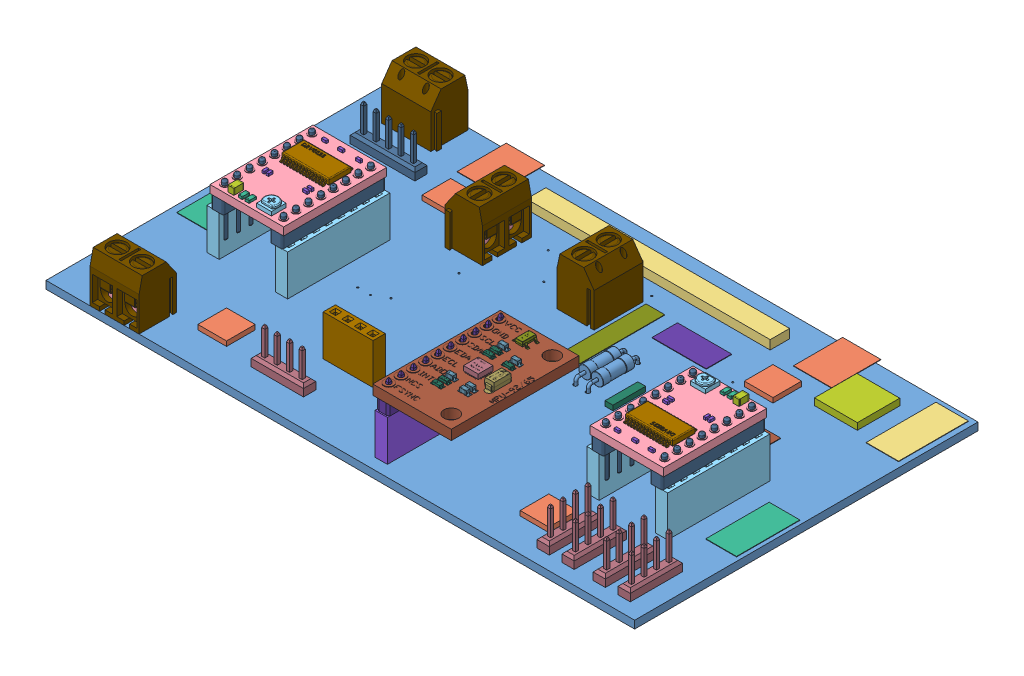
SolidWorks assembly RILey_PCB, configuration Default. Lengths in mm.
Overall size (120 19.05 71.04).
92 component instances, 36 part files, 22 mates.
Components (placement in the parent):
- RILey_PCB.step-1: RILey_PCB.step [Default] at (-11.3624 54.5013 128.2539) x (1 0 0) z (0 1 0) size (120 71.04 11.3)
  - PCB Component.step-1: PCB Component.step [Default] at origin size (120 71.04 11.3)
    - Board.step-1: Board.step [Default] at origin size (120 70 1.57)
    - 0026604020.step-1: 0026604020.step [Default] at (95.25 66.04 1.57) size (7.77 10.01 0.1)
    - 0026604020.step-2: 0026604020.step [Default] at (26.67 66.04 1.57) size (7.77 10.01 0.1)
    - 2540-.step-1: 2540-.step [Default] at (61.27 63.5 1.57) size (49.68 3.96 1.83)
    - W237-102.step-1: W237-102.step [Default] at (11.481 64.491 1.57) x (-1 0 0) z (0 0 1) size (6.7 3.4 2.59)
    - W237-102.step-2: W237-102.step [Default] at (13.97 5.08 1.57) size (6.7 3.4 2.59)
    - W237-102.step-3: W237-102.step [Default] at (59.588 52.07 1.57) x (0 1 0) z (0 0 1) size (6.7 3.4 2.59)
    - W237-102.step-4: W237-102.step [Default] at (39.37 52.07 1.57) x (0 -1 0) z (0 0 1) size (6.7 3.4 2.59)
    - FE08-1_3D.step-1: FE08-1_3D.step [Default] at (26.67 31.75 1.57) x (0 1 0) z (0 0 1) size (20.82 2.5 11.3)
    - FE08-1_3D.step-2: FE08-1_3D.step [Default] at (12.7 31.75 1.57) x (0 1 0) z (0 0 1) size (20.82 2.5 11.3)
    - FE08-1_3D.step-3: FE08-1_3D.step [Default] at (93.98 27.94 1.57) x (0 -1 0) z (0 0 1) size (20.82 2.5 11.3)
    - FE08-1_3D.step-4: FE08-1_3D.step [Default] at (107.95 27.94 1.57) x (0 -1 0) z (0 0 1) size (20.82 2.5 11.3)
    - B4B-XH-A_LF__SN_.step-1: B4B-XH-A_LF__SN_.step [Default] at (5.08 27.94 1.57) x (0 1 0) z (0 0 1) size (12.9 6.25 0.1)
    - B4B-XH-A_LF__SN_.step-2: B4B-XH-A_LF__SN_.step [Default] at (115.57 31.75 1.57) x (0 -1 0) z (0 0 1) size (12.9 6.25 0.1)
    - 733980-62.step-1: 733980-62.step [Default] at (106.68 66.04 1.57) x (-1 0 0) z (0 0 1) size (8.75 8.65 1.36)
    - FE10-1_3D.step-1: FE10-1_3D.step [Default] at (66.04 15.259 1.57) x (0 -1 0) z (0 0 1) size (25.9 2.5 11.3)
    - FE04-1.step-1: FE04-1.step [Default] at (51.003 15.646 1.57) x (-1 0 0) z (0 0 1) size (10.16 2.5 11.3)
    - MA05-1_SMALLPAD.step-1: MA05-1_SMALLPAD.step [Default] at (13.97 55.88 1.57) x (-1 0 0) z (0 0 1) size (13.2 2.5 11)
    - 100uF.step-1: 100uF.step [Default] at (10.16 46.99 1.57) x (-1 0 0) z (0 0 1) size (7.55 7.55 0.1)
    - 100uF.step-2: 100uF.step [Default] at (97.79 43.18 1.57) size (7.55 7.55 0.1)
    - PTS18126V260.step-1: PTS18126V260.step [Default] at (62.23 40.64 0) x (0 1 0) z (0 0 -1) size (5.95 3.93 0.1)
    - MA04-1_SMALLPAD.step-1: MA04-1_SMALLPAD.step [Default] at (99.06 7.62 1.57) x (0 -1 0) z (0 0 1) size (10.66 2.5 11)
    - MA04-1_SMALLPAD.step-2: MA04-1_SMALLPAD.step [Default] at (104.14 7.62 1.57) x (0 -1 0) z (0 0 1) size (10.66 2.5 11)
    - MA04-1_SMALLPAD.step-3: MA04-1_SMALLPAD.step [Default] at (110.49 7.62 1.57) x (0 -1 0) z (0 0 1) size (10.66 2.5 11)
    - MA04-1_SMALLPAD.step-4: MA04-1_SMALLPAD.step [Default] at (115.57 7.62 1.57) x (0 -1 0) z (0 0 1) size (10.66 2.5 11)
    - MA04-1_SMALLPAD.step-5: MA04-1_SMALLPAD.step [Default] at (42.012 6.401 1.57) x (-1 0 0) z (0 0 1) size (10.66 2.5 11)
    - 1uF.step-1: 1uF.step [Default] at (85.09 36.83 1.57) x (0 -1 0) z (0 0 1) size (4.14 1.6 1.07)
    - 47uF.step-1: 47uF.step [Default] at (80.01 38.1 1.57) x (0 -1 0) z (0 0 1) size (6.68 1.6 0.99)
    - SA5.0A-E3_54.step-1: SA5.0A-E3_54.step [Default] at (67.31 55.88 1.57) x (0 -1 0) z (0 0 1) size (21.18 3.8 0.1)
    - IRF9530NPBF.step-1: IRF9530NPBF.step [Default] at (74.93 53.34 1.57) size (11.04 5.19 0.1)
    - BCM857BS,115.step-1: BCM857BS,115.step [Default] at (78.74 48.26 0) x (1 0 0) z (0 0 -1) size (3.4 2.7 0.1)
    - 10k.step-1: 10k.step [Default] at (74.93 40.64 1.57) x (0 1 0) z (0 0 1) size (10.6 2.5 4.42)
    - 10k.step-2: 10k.step [Default] at (72.39 40.64 1.57) x (0 1 0) z (0 0 1) size (10.6 2.5 4.42)
    - 2,8.step-1: 2,8.step [Default] at (27.15 9.65 1.57) size (5.84 5.84 0.97)
    - 2,8.step-2: 2,8.step [Default] at (92.85 55.35 1.57) size (5.84 5.84 0.97)
    - 2,8.step-3: 2,8.step [Default] at (27.15 55.35 1.57) size (5.84 5.84 0.97)
    - 2,8.step-4: 2,8.step [Default] at (92.85 9.65 1.57) size (5.84 5.84 0.97)
    - 1101M2S3CQE2.step-1: 1101M2S3CQE2.step [Default] at (115.621 62.763 1.57) size (6.6 14.23 0.1)
- DRV 8825 With Headers Assem-1: DRV 8825 With Headers Assem [Default] at (18.6208 50.4495 104.6201) x (0 0 -1) z (0 1 0) size (21 15 10.9)
  - PCB-1: PCB [Default] at (8.1162 10.2982 16.4218) size (21 15 1.8)
  - SMD Pot-1: SMD Pot [Default] at (-0.2134 7.4613 18.0218) x (0 -1 0) z (0 0 1) size (3 3 1.3)
  - 0603 Resistor-1: 0603 Resistor [Default] at (-1.0068 10.8561 18.0218) size (1.5 0.8 0.5)
  - 0603 Resistor-2: 0603 Resistor [Default] at (-1.0286 12.2306 18.0218) size (1.5 0.8 0.5)
  - 0805 Capacitor-1: 0805 Capacitor [Default] at (-0.8941 14.0417 18.0218) size (2 1.25 1.25)
  - 0402 Resistor-1: 0402 Resistor [Default] at (16.8896 6.6863 18.0218) x (0 -1 0) z (0 0 1) size (1 0.68 0.66)
  - 0402 Resistor-2: 0402 Resistor [Default] at (16.8896 10.308 18.0218) x (0 -1 0) z (0 0 1) size (1 0.68 0.66)
  - 0402 Resistor-3: 0402 Resistor [Default] at (16.8896 13.6408 18.0218) x (0 -1 0) z (0 0 1) size (1 0.68 0.66)
  - 0402 Resistor-4: 0402 Resistor [Default] at (6.8882 6.5987 18.0218) x (0 -1 0) z (0 0 1) size (1 0.68 0.66)
  - 0402 Resistor-5: 0402 Resistor [Default] at (5.9719 6.5987 18.0218) x (0 -1 0) z (0 0 1) size (1 0.68 0.66)
  - 0402 Resistor-6: 0402 Resistor [Default] at (5.456 14.3274 18.0218) size (1 0.68 0.66)
  - 0402 Resistor-7: 0402 Resistor [Default] at (5.456 13.4855 18.0218) size (1 0.68 0.66)
  - DRV8825 IC-1: DRV8825 IC [Default] at (11.7347 10.2312 18.0218) x (0 -1 0) z (0 0 1) size (9.6 6.2 1.2)
  - 8 pin Header-1: 8 pin Header [Default] at (8.1162 16.2982 13.9218) size (21 2.5 10.5)
  - 8 pin Header-2: 8 pin Header [Default] at (8.1162 4.2982 13.9218) size (21 2.5 10.5)
- DRV 8825 With Headers Assem-2: DRV 8825 With Headers Assem [Default] at (79.3044 50.4495 92.1976) x (0 0 1) z (0 1 0) size (21 15 10.9)
  - PCB-1: PCB [Default] at (8.1162 10.2982 16.4218) size (21 15 1.8)
  - SMD Pot-1: SMD Pot [Default] at (-0.2134 7.4613 18.0218) x (0 -1 0) z (0 0 1) size (3 3 1.3)
  - 0603 Resistor-1: 0603 Resistor [Default] at (-1.0068 10.8561 18.0218) size (1.5 0.8 0.5)
  - 0603 Resistor-2: 0603 Resistor [Default] at (-1.0286 12.2306 18.0218) size (1.5 0.8 0.5)
  - 0805 Capacitor-1: 0805 Capacitor [Default] at (-0.8941 14.0417 18.0218) size (2 1.25 1.25)
  - 0402 Resistor-1: 0402 Resistor [Default] at (16.8896 6.6863 18.0218) x (0 -1 0) z (0 0 1) size (1 0.68 0.66)
  - 0402 Resistor-2: 0402 Resistor [Default] at (16.8896 10.308 18.0218) x (0 -1 0) z (0 0 1) size (1 0.68 0.66)
  - 0402 Resistor-3: 0402 Resistor [Default] at (16.8896 13.6408 18.0218) x (0 -1 0) z (0 0 1) size (1 0.68 0.66)
  - 0402 Resistor-4: 0402 Resistor [Default] at (6.8882 6.5987 18.0218) x (0 -1 0) z (0 0 1) size (1 0.68 0.66)
  - 0402 Resistor-5: 0402 Resistor [Default] at (5.9719 6.5987 18.0218) x (0 -1 0) z (0 0 1) size (1 0.68 0.66)
  - 0402 Resistor-6: 0402 Resistor [Default] at (5.456 14.3274 18.0218) size (1 0.68 0.66)
  - 0402 Resistor-7: 0402 Resistor [Default] at (5.456 13.4855 18.0218) size (1 0.68 0.66)
  - DRV8825 IC-1: DRV8825 IC [Default] at (11.7347 10.2312 18.0218) x (0 -1 0) z (0 0 1) size (9.6 6.2 1.2)
  - 8 pin Header-1: 8 pin Header [Default] at (8.1162 16.2982 13.9218) size (21 2.5 10.5)
  - 8 pin Header-2: 8 pin Header [Default] at (8.1162 4.2982 13.9218) size (21 2.5 10.5)
- MPU9250.STEP-2: MPU9250.STEP [Default] at (87.1776 67.9346 116.1747) x (0 0 1) z (-1 0 0) size (26 3.91 16)
  - PCB.STEP-1: PCB.STEP [Default] at (-2.9998 1.0768 26) size (26 2.2 16)
  - C2.STEP-1: C2.STEP [Default] at (-2.4989 2.0768 21) x (0 0 -1) z (1 0 0) size (2 1.81 5.01)
  - MP92.STEP-1: MP92.STEP [Default] at (-2.9998 1.0968 25.5) x (0 0 -1) z (1 0 0) size (3.29 1.01 3.29)
  - C1_Predeterminado_Como mecanizada_.STEP-1: C1_Predeterminado_Como mecanizada_.STEP [Default] at (2.1384 1.0968 23.0905) x (0 0 1) z (-1 0 0) size (2.2 0.83 0.9)
  - C1_Predeterminado_Como mecanizada_.STEP-2: C1_Predeterminado_Como mecanizada_.STEP [Default] at (0.9102 1.0968 27.1044) x (0 0 1) z (-1 0 0) size (2.2 0.83 0.9)
  - C1_Predeterminado_Como mecanizada_.STEP-3: C1_Predeterminado_Como mecanizada_.STEP [Default] at (0.9102 1.0968 23.0905) x (0 0 1) z (-1 0 0) size (2.2 0.83 0.9)
  - C1_Predeterminado_Como mecanizada_.STEP-4: C1_Predeterminado_Como mecanizada_.STEP [Default] at (-8.3098 1.0968 23.0905) x (0 0 1) z (-1 0 0) size (2.2 0.83 0.9)
  - C1_Predeterminado_Como mecanizada_.STEP-5: C1_Predeterminado_Como mecanizada_.STEP [Default] at (-9.7098 1.0968 27.1044) x (0 0 1) z (-1 0 0) size (2.2 0.83 0.9)
  - R1.STEP-1: R1.STEP [Default] at (3.5484 1.1168 27.2144) x (0 0 -1) z (1 0 0) size (2.2 0.47 0.9)
  - R1.STEP-2: R1.STEP [Default] at (2.1484 1.1168 27.2144) x (0 0 -1) z (1 0 0) size (2.2 0.47 0.9)
  - R1.STEP-3: R1.STEP [Default] at (-6.8998 1.1168 23.2005) x (0 0 -1) z (1 0 0) size (2.2 0.47 0.9)
  - R1.STEP-4: R1.STEP [Default] at (-8.2998 1.1168 27.2144) x (0 0 -1) z (1 0 0) size (2.2 0.47 0.9)
  - R1.STEP-5: R1.STEP [Default] at (-6.8998 1.1168 27.2144) x (0 0 -1) z (1 0 0) size (2.2 0.47 0.9)
  - V1.STEP-1: V1.STEP [Default] at (-13.0785 1.5868 25.9) size (2.9 0.96 3.2)
- PinHeader10row-1: PinHeader10row [Default] at (53.4076 66.9113 102.8349) x (0 0 -1) z (-1 0 0) size (25.4 11.54 2.54)
- DG301-5.0-02-1: DG301-5.0-02 [Default] at (0.1076 56.0713 125.1439) x (1 0 0) z (0 1 0) size (10.6 7.6 14.3)
- DG301-5.0-02-2: DG301-5.0-02 [Default] at (27.4376 56.0713 78.6839) x (0 0 -1) z (0 1 0) size (10.6 7.6 14.3)
- DG301-5.0-02-3: DG301-5.0-02 [Default] at (48.7956 56.0713 73.6839) x (0 0 1) z (0 1 0) size (10.6 7.6 14.3)
- DG301-5.0-02-4: DG301-5.0-02 [Default] at (2.6186 56.0713 61.7929) x (-1 0 0) z (0 1 0) size (10.6 7.6 14.3)
Mates (geometry in assembly coordinates):
- Coincident1: coincident anti-aligned: plane of RILey_PCB.step-1/PCB Component.step-1/FE08-1_3D.step-1 through (15.3076 64.3713 96.5039) normal (0 1 0); plane of DRV 8825 With Headers Assem-1/8 pin Header-2 through (14.3226 64.3713 96.5039) normal (0 -1 0)
- Coincident2: coincident anti-aligned: plane of RILey_PCB.step-1/PCB Component.step-1/FE08-1_3D.step-4 through (96.5876 64.3713 100.3139) normal (0 1 0); plane of DRV 8825 With Headers Assem-2/8 pin Header-2 through (83.6026 64.3713 100.3139) normal (0 -1 0)
- Width1: width aligned: plane of DRV 8825 With Headers Assem-1/PCB-1 through (0.8226 68.4713 107.0039) normal (0 0 1); plane of DRV 8825 With Headers Assem-1/PCB-1 through (0.8226 68.4713 86.0039) normal (0 0 -1); plane of RILey_PCB.step-1/PCB Component.step-1/FE08-1_3D.step-1 through (15.3076 60.2213 106.9139) normal (0 0 1); plane of RILey_PCB.step-1/PCB Component.step-1/FE08-1_3D.step-1 through (15.3076 60.2213 86.0939) normal (0 0 -1)
- Width3: width aligned: plane of DRV 8825 With Headers Assem-1/PCB-1 through (0.8226 68.4713 107.0039) normal (-1 0 0); plane of DRV 8825 With Headers Assem-1/PCB-1 through (15.8226 68.4713 107.0039) normal (1 0 0); plane of RILey_PCB.step-1/PCB Component.step-1/FE08-1_3D.step-2 through (0.0876 60.2213 96.5039) normal (-1 0 0); plane of RILey_PCB.step-1/PCB Component.step-1/FE08-1_3D.step-1 through (16.5576 60.2213 96.5039) normal (1 0 0)
- Width4: width anti-aligned: plane of DRV 8825 With Headers Assem-2/PCB-1 through (97.1026 68.4713 110.8139) normal (0 0 1); plane of DRV 8825 With Headers Assem-2/PCB-1 through (97.1026 68.4713 89.8139) normal (0 0 -1); plane of RILey_PCB.step-1/PCB Component.step-1/FE08-1_3D.step-4 through (96.5876 60.2213 89.9039) normal (0 0 -1); plane of RILey_PCB.step-1/PCB Component.step-1/FE08-1_3D.step-4 through (96.5876 60.2213 110.7239) normal (0 0 1)
- Width5: width aligned: plane of DRV 8825 With Headers Assem-2/PCB-1 through (97.1026 68.4713 89.8139) normal (1 0 0); plane of DRV 8825 With Headers Assem-2/PCB-1 through (82.1026 68.4713 89.8139) normal (-1 0 0); plane of RILey_PCB.step-1/PCB Component.step-1/FE08-1_3D.step-4 through (97.8376 60.2213 100.3139) normal (1 0 0); plane of RILey_PCB.step-1/PCB Component.step-1/FE08-1_3D.step-3 through (81.3676 60.2213 100.3139) normal (-1 0 0)
- ProfileCenter1: profile center = 1.85 mm anti-aligned: plane of PinHeader10row-1 through (53.4076 58.3713 125.6949) normal (0 -1 0); plane of RILey_PCB.step-1/PCB Component.step-1/FE10-1_3D.step-1 through (54.6776 60.2213 124.4249) normal (0 1 0)
- Concentric2: concentric aligned: circle of RILey_PCB.step-1/PCB Component.step-1/Board.step-1; cylinder of MPU9250.STEP-2/PCB.STEP-1 through (54.6776 67.0113 124.4249) axis (0 1 0) radius 0.5
- Parallel2: parallel aligned: plane of RILey_PCB.step-1/PCB Component.step-1/FE10-1_3D.step-1 through (54.6776 60.2213 100.0449) normal (0 0 -1); plane of MPU9250.STEP-2/PCB.STEP-1 through (61.1776 67.0113 100.1749) normal (0 0 -1)
- Coincident4: coincident anti-aligned: plane of MPU9250.STEP-2/PCB.STEP-1 through (61.1776 66.9113 113.1749) normal (0 -1 0); plane of PinHeader10row-1 through (53.4076 66.9113 105.3749) normal (0 1 0)
- Coincident174: coincident anti-aligned: plane of RILey_PCB.step-1/PCB Component.step-1/Board.step-1 through (48.6376 56.0713 93.2539) normal (0 1 0); plane of DG301-5.0-02-1 through (-2.3924 56.0713 128.2439) normal (0 -1 0)
- Width24: width anti-aligned: plane of DG301-5.0-02-1; plane of RILey_PCB.step-1/PCB Component.step-1/W237-102.step-2; plane of DG301-5.0-02-1 through (-0.7433 56.0713 126.1457) normal (0 0 1); plane of RILey_PCB.step-1/PCB Component.step-1/W237-102.step-2 through (5.9585 56.0713 122.7421) normal (0 0 -1)
- Width26: width aligned: plane of DG301-5.0-02-1; plane of RILey_PCB.step-1/PCB Component.step-1/W237-102.step-2; plane of DG301-5.0-02-1 through (5.9585 56.0713 126.1457) normal (1 0 0); plane of RILey_PCB.step-1/PCB Component.step-1/W237-102.step-2 through (-0.7433 56.0713 122.7421) normal (-1 0 0)
- Width18: width anti-aligned: plane of DG301-5.0-02-2 through (27.4376 56.0713 81.1839) normal (0 0 1); plane of RILey_PCB.step-1/PCB Component.step-1/W237-102.step-4 through (27.4376 56.0713 71.1839) normal (0 0 -1); plane of DG301-5.0-02-2 through (28.4394 56.0713 72.833) normal (0 0 -1); plane of RILey_PCB.step-1/PCB Component.step-1/W237-102.step-4 through (25.0358 56.0713 79.5348) normal (0 0 1)
- Width19: width aligned: plane of DG301-5.0-02-2 through (30.5376 56.0713 71.1839) normal (1 0 0); plane of RILey_PCB.step-1/PCB Component.step-1/W237-102.step-4 through (22.9376 63.0713 71.1839) normal (-1 0 0); plane of DG301-5.0-02-2 through (28.4394 56.0713 79.5348) normal (1 0 0); plane of RILey_PCB.step-1/PCB Component.step-1/W237-102.step-4 through (25.0358 56.0713 72.833) normal (-1 0 0)
- Coincident175: coincident anti-aligned: plane of RILey_PCB.step-1/PCB Component.step-1/Board.step-1 through (48.6376 56.0713 93.2539) normal (0 1 0); plane of DG301-5.0-02-2 through (22.9376 56.0713 71.1839) normal (0 -1 0)
- Width20: width aligned: plane of DG301-5.0-02-3; plane of RILey_PCB.step-1/PCB Component.step-1/W237-102.step-3; plane of DG301-5.0-02-3 through (51.1974 56.0713 72.833) normal (0 0 -1); plane of RILey_PCB.step-1/PCB Component.step-1/W237-102.step-3 through (47.7938 56.0713 79.5348) normal (0 0 1)
- Width21: width aligned: plane of DG301-5.0-02-3 through (53.2956 56.0713 71.1839) normal (1 0 0); plane of RILey_PCB.step-1/PCB Component.step-1/W237-102.step-3 through (45.6956 63.0713 71.1839) normal (-1 0 0); plane of DG301-5.0-02-3 through (47.7938 56.0713 72.833) normal (-1 0 0); plane of RILey_PCB.step-1/PCB Component.step-1/W237-102.step-3 through (51.1974 56.0713 79.5348) normal (1 0 0)
- Coincident176: coincident anti-aligned: plane of RILey_PCB.step-1/PCB Component.step-1/Board.step-1 through (48.6376 56.0713 93.2539) normal (0 1 0); plane of DG301-5.0-02-3 through (45.6956 56.0713 71.1839) normal (0 -1 0)
- Width22: width aligned: plane of DG301-5.0-02-4 through (-4.8814 56.0713 58.6929) normal (0 0 -1); plane of RILey_PCB.step-1/PCB Component.step-1/W237-102.step-1 through (-4.8814 63.0713 66.2929) normal (0 0 1); plane of DG301-5.0-02-4 through (3.4695 56.0713 60.7911) normal (0 0 -1); plane of RILey_PCB.step-1/PCB Component.step-1/W237-102.step-1 through (-3.2323 56.0713 64.1947) normal (0 0 1)
- Width23: width anti-aligned: plane of DG301-5.0-02-4 through (-4.8814 56.0713 61.7929) normal (-1 0 0); plane of RILey_PCB.step-1/PCB Component.step-1/W237-102.step-1 through (5.1186 56.0713 61.7929) normal (1 0 0); plane of DG301-5.0-02-4 through (3.4695 56.0713 64.1947) normal (1 0 0); plane of RILey_PCB.step-1/PCB Component.step-1/W237-102.step-1 through (-3.2323 56.0713 60.7911) normal (-1 0 0)
- Coincident177: coincident anti-aligned: plane of RILey_PCB.step-1/PCB Component.step-1/Board.step-1 through (48.6376 56.0713 93.2539) normal (0 1 0); plane of DG301-5.0-02-4 through (-4.8814 56.0713 66.2929) normal (0 -1 0)
